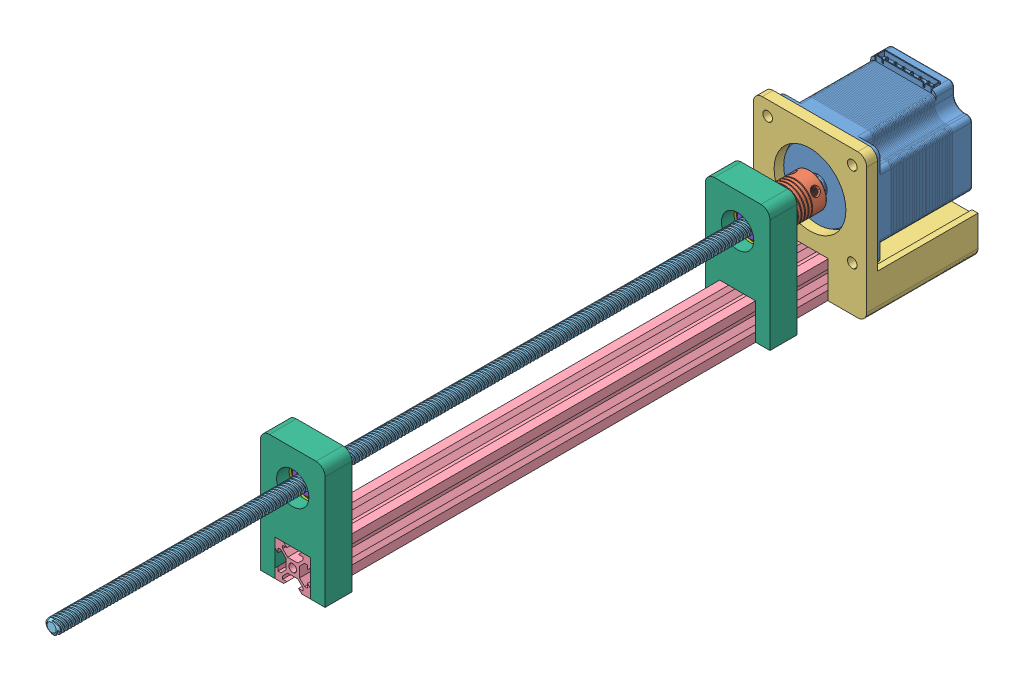
SolidWorks assembly EjeBase, configuration Predeterminado. Lengths in mm.
Overall size (63.14 80.17 487.23).
17 component instances, 9 part files, 15 mates.
Components (placement in the parent):
- Nema 23-1: Nema 23 [Default] at (-11.5289 2.714 38.3) size (56.4 59.4 76.6)
- Coupler 6.35-8mm-1: Coupler 6.35-8mm [Default] at (-11.5289 2.714 113.0023) x (0.819898 0.57251 0) z (0 0 1) size (19.34 19.34 25)
- SoporteNEMA-1-1: SoporteNEMA-1 [Predeterminado] at (12.0411 26.284 100.3) x (-1 0 0) z (0 0 -1) size (63.14 80.17 62)
- BoschBase-1: BoschBase [Predeterminado] at (-21.6289 -25.886 38.3) size (20 20 350)
- VarillaBase-1: VarillaBase [Default] at (-11.5289 2.714 522.6863) x (0.999103 -0.042354 0) z (0 0 1) size (8.33 8.33 405.47)
- TopeVarilla-1: TopeVarilla [Predeterminado] at (-27.6485 -16.346 448.8) x (-1 0 0) z (0 0 -1) size (36 68 15)
  - SoporteVarilla1-1: SoporteVarilla1 [Predeterminado] at (-26.0197 -9.54 60.5) size (36 68 15)
  - skf_bearing_609_2-1: skf_bearing_609_2 [Default] at (-16.0197 19.06 74.5) x (0 0 -1) z (1 0 0) size (7 24 24)
    - skf_bearing_609_2_01-1: skf_bearing_609_2_01 [Default] at origin size (7 24 24)
    - skf_bearing_609_2_02-1: skf_bearing_609_2_02 [Default] at origin size (7 14.45 14.45)
    - skf_bearing_609_2_03-1: skf_bearing_609_2_03 [Default] at origin size (3.97 20.97 20.97)
- TopeVarilla-2: TopeVarilla [Predeterminado] at (-27.6485 -16.346 201.0023) x (-1 0 0) z (0 0 -1) size (36 68 15)
  - SoporteVarilla1-1: SoporteVarilla1 [Predeterminado] at (-26.0197 -9.54 60.5) size (36 68 15)
  - skf_bearing_609_2-1: skf_bearing_609_2 [Default] at (-16.0197 19.06 74.5) x (0 0 -1) z (1 0 0) size (7 24 24)
    - skf_bearing_609_2_01-1: skf_bearing_609_2_01 [Default] at origin size (7 24 24)
    - skf_bearing_609_2_02-1: skf_bearing_609_2_02 [Default] at origin size (7 14.45 14.45)
    - skf_bearing_609_2_03-1: skf_bearing_609_2_03 [Default] at origin size (3.97 20.97 20.97)
Mates (geometry in assembly coordinates):
- Concéntrica1: concentric anti-aligned: cylinder of Nema 23-1 through (-11.5289 2.714 99.9) axis (0 0 -1) radius 3.175; cylinder of Coupler 6.35-8mm-1 through (-11.5289 2.714 115.5023) axis (0 0 1) radius 3.175
- Coincidente1: coincident anti-aligned: plane of Nema 23-1 through (-35.7289 -21.486 94.3) normal (0 0 1); plane of SoporteNEMA-1-1 through (12.0411 26.284 94.3) normal (0 0 -1)
- Coincidente2: coincident anti-aligned: plane of Nema 23-1 through (4.1711 -25.486 49.1) normal (0 -1 0); plane of SoporteNEMA-1-1 through (12.0411 -25.486 38.3) normal (0 1 0)
- Concéntrica2: concentric anti-aligned: cylinder of Nema 23-1 through (-35.0989 26.284 94.3) axis (0 0 -1) radius 2.5; cylinder of SoporteNEMA-1-1 through (-35.0989 26.284 94.3) axis (0 0 1) radius 2.7
- Coincidente3: coincident anti-aligned: plane of SoporteNEMA-1-1 through (-21.6289 26.284 38.3) normal (1 0 0); plane of BoschBase-1 through (-21.6289 -25.886 388.3) normal (-1 0 0)
- Coincidente4: coincident aligned: plane of SoporteNEMA-1-1 through (12.0411 -45.886 100.3) normal (0 -1 0); plane of BoschBase-1 through (-21.6289 -45.886 388.3) normal (0 -1 0)
- Coincidente5: coincident aligned: plane of SoporteNEMA-1-1 through (12.0411 26.284 38.3) normal (0 0 -1); plane of BoschBase-1 through (-21.6289 -25.886 38.3) normal (0 0 -1)
- Concéntrica4: concentric aligned: circle of Coupler 6.35-8mm-1; circle of VarillaBase-1
- Coincidente16: coincident anti-aligned: plane of BoschBase-1 through (-21.6289 -25.886 388.3) normal (-1 0 0); plane of TopeVarilla-1/SoporteVarilla1-1 through (-21.6289 -25.886 373.3) normal (1 0 0)
- Coincidente17: coincident aligned: plane of BoschBase-1 through (-21.6289 -25.886 388.3) normal (0 0 1); plane of TopeVarilla-1/SoporteVarilla1-1 through (-1.6289 -25.886 388.3) normal (0 0 1)
- Coincidente18: coincident aligned: plane of BoschBase-1 through (-21.6289 -45.886 388.3) normal (0 -1 0); plane of TopeVarilla-1/SoporteVarilla1-1 through (-1.6289 -45.886 373.3) normal (0 -1 0)
- Bloquear2: lock: unknown of Nema 23-1; unknown of Coupler 6.35-8mm-1
- Coincidente23: coincident: plane of BoschBase-1 through (-1.6289 -25.886 388.3) normal (1 0 0); plane of TopeVarilla-2/SoporteVarilla1-1 through (-1.6289 -25.886 125.5023) normal (-1 0 0)
- Coincidente24: coincident: plane of BoschBase-1 through (-21.6289 -45.886 388.3) normal (0 -1 0); plane of TopeVarilla-2/SoporteVarilla1-1 through (-1.6289 -45.886 125.5023) normal (0 -1 0)
- Coincidente25: coincident anti-aligned: plane of Coupler 6.35-8mm-1 through (-11.5289 2.714 125.5023) normal (0 0 1); plane of TopeVarilla-2/SoporteVarilla1-1 through (-1.6289 -25.886 125.5023) normal (0 0 -1)
